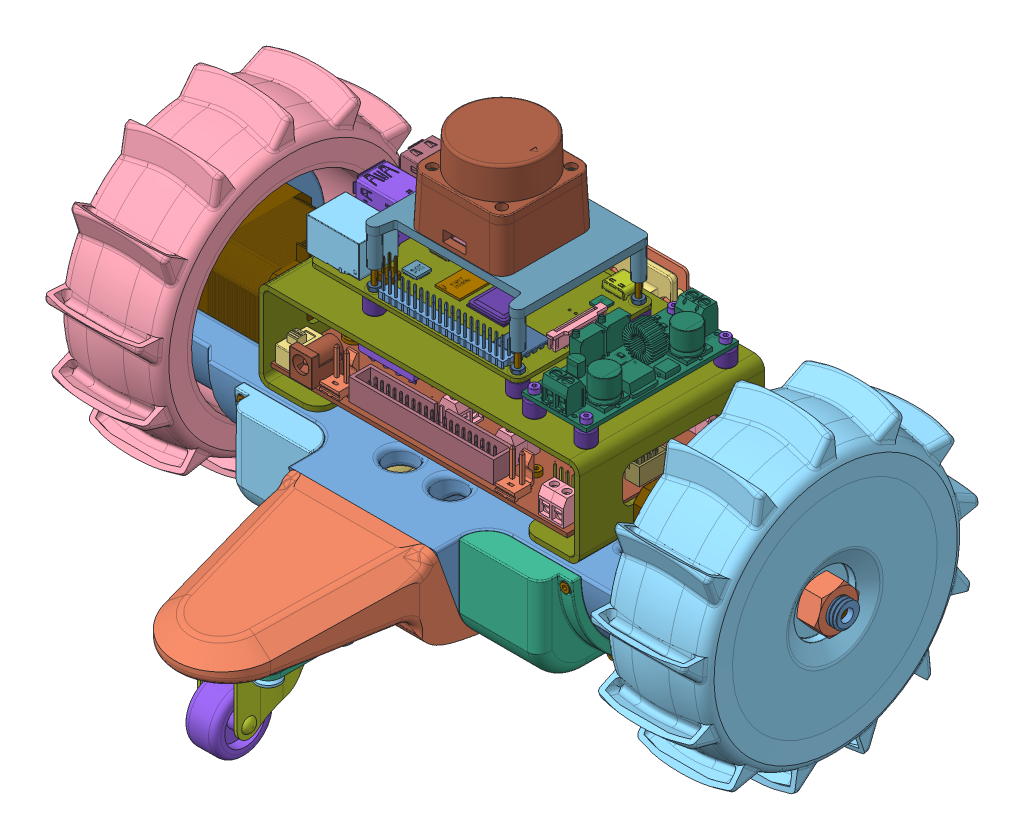
SolidWorks assembly RILeyV2_Assembly, configuration Default. Lengths in mm. (continued)
Components (placement in the parent): (continued)
- hex nut style 1 gradeab_iso-8: hex nut style 1 gradeab_iso [ISO - 4032 - M3 - W - C] at (300.5332 207.7689 553.3328) x (1 0 0) z (0 1 0) size (5.5 6.35 2.4)
- socket countersunk head screw_iso-2: socket countersunk head screw_iso [ISO 10642 - M5 x 10 - 10C] at (238.0332 177.1861 610.0431) x (0 1 0) z (-0.9954 0 -0.095805) size (10 9.43 9.43)
- socket countersunk head screw_iso-3: socket countersunk head screw_iso [ISO 10642 - M5 x 10 - 10C] at (238.0332 177.1861 639.0431) x (0 1 0) z (-0.549026 0 0.835805) size (10 9.43 9.43)
- socket countersunk head screw_iso-4: socket countersunk head screw_iso [ISO 10642 - M5 x 10 - 10C] at (267.0332 177.1861 639.0431) x (0 1 0) z (-0.752778 0 -0.658274) size (10 9.43 9.43)
- socket countersunk head screw_iso-5: socket countersunk head screw_iso [ISO 10642 - M5 x 10 - 10C] at (267.0332 177.1861 610.0431) x (0 1 0) z (-0.538139 0 0.842856) size (10 9.43 9.43)
Mates (geometry in assembly coordinates):
- Coincident1: coincident aligned: plane of MiddlepartV2-1 through (252.5332 203.3689 525.8328) normal (0 1 0); plane of MiddlepartTailV2-1 through (282.5332 203.3689 577.1871) normal (0 1 0)
- Coincident4: coincident anti-aligned: line of MiddlepartV2-1 through (223.5332 203.3689 586.6171) axis (1 0 0); line of MiddlepartTailV2-1 through (278.0554 203.3689 586.6171) axis (-1 0 0)
- Width1: width anti-aligned: plane of MiddlepartTailV2-1 through (283.4552 145.3689 587.849) normal (0.985029 0 0.172389); plane of MiddlepartV2-1 through (219.8281 145.3689 577.6605) normal (-0.985029 0 0.172389); plane of MiddlepartTailV2-1 through (282.5332 203.3689 670.8328) normal (1 0 0); plane of MiddlepartV2-1 through (222.5332 203.3689 670.8328) normal (-1 0 0)
- Coincident6: coincident anti-aligned: plane of swifflewheel-1 through (31.0041 112.5645 302.2353) normal (0 1 0); plane of MiddlepartTailV2-1 through (222.5332 182.3689 577.1871) normal (0 -1 0)
- Width2: width aligned: plane of swifflewheel-1 through (26.0041 112.5645 302.2353) normal (-1 0 0); plane of MiddlepartTailV2-1 through (66.0041 112.5645 302.2353) normal (1 0 0); plane of swifflewheel-1 through (283.4552 145.3689 587.849) normal (0.985029 0 0.172389); plane of MiddlepartTailV2-1 through (219.8281 145.3689 577.6605) normal (-0.985029 0 0.172389)
- Coincident8: coincident: plane of swifflewheel-1 through (31.0041 112.5645 307.2353) normal (0 0 1); line of MiddlepartTailV2-1 through (231.5332 185.8689 644.5431) axis (0 1 0)
- Concentric1: concentric aligned: circle of swifflewheel-1; circle of swifflewheelMid-1
- Coincident9: coincident anti-aligned: plane of swifflewheel-1 through (31.0041 109.0645 302.2353) normal (0 -1 0); plane of swifflewheelMid-1 through (46.0041 109.0645 287.2353) normal (0 1 0)
- Concentric2: concentric aligned: cylinder of swifflewheelMid-1 through (58.5007 88.5361 300.0351) axis (-0.952407 0 0.30483) radius 1.5; cylinder of swifflewheelwheel-1 through (-895.8822 88.5361 605.4977) axis (-0.952407 0 0.30483) radius 1.5
- Width3: width anti-aligned: plane of swifflewheelMid-1 through (36.5271 75.0645 279.7688) normal (0.952407 0 -0.30483); plane of swifflewheelwheel-1 through (49.3846 75.0645 275.6536) normal (-0.952407 0 0.30483); plane of swifflewheelMid-1 through (45.0365 87.5545 305.5354) normal (-0.952407 0 0.30483); plane of swifflewheelwheel-1 through (57.4178 87.5545 301.5726) normal (0.952407 0 -0.30483)
- Concentric3: concentric anti-aligned: circle of MiddlepartV2-1; circle of ReelyBuggyWheel_Left-1
- Concentric4: concentric anti-aligned: circle of MiddlepartV2-1; circle of ReelyBuggyWheel_Right-1
- Coincident12: coincident anti-aligned: plane of MiddlepartV2-1 through (367.5332 203.3689 525.8328) normal (1 0 0); plane of ReelyBuggyWheel_Right-1 through (161.0041 133.5645 188.525) normal (-1 0 0)
- Coincident13: coincident anti-aligned: plane of MiddlepartV2-1 through (137.5332 203.3689 525.8328) normal (-1 0 0); plane of ReelyBuggyWheel_Left-1 through (-68.9959 133.5645 188.525) normal (1 0 0)
- Concentric6: concentric aligned: cylinder of MiddlepartV2-1 through (300.5332 190.4192 498.3328) axis (0 1 0) radius 1.75; cylinder of 3rdFloor_Sheetmetal-1 through (94.0041 128.6147 161.025) axis (0 1 0) radius 1.75
- Coincident14: coincident anti-aligned: plane of MiddlepartV2-1 through (252.5332 203.3689 525.8328) normal (0 1 0); plane of 3rdFloor_Sheetmetal-1 through (46.0041 133.5645 188.525) normal (0 -1 0)
- Concentric7: concentric aligned: cylinder of MiddlepartV2-1 through (204.5332 190.4192 498.3328) axis (0 1 0) radius 1.75; cylinder of 3rdFloor_Sheetmetal-1 through (-1.9959 128.6147 161.025) axis (0 1 0) radius 1.75
- Concentric8: concentric aligned: cylinder of MiddlepartTailV2-1 through (238.0332 207.3041 610.0431) axis (0 -1 0) radius 2.3; cylinder of SwivelWheel-1/SwivelWheelBase-1 through (238.0332 182.3689 610.0431) axis (0 -1 0) radius 2.65
- Concentric10: concentric aligned: cylinder of MiddlepartTailV2-1 through (267.0332 207.3041 610.0431) axis (0 -1 0) radius 2.3; cylinder of SwivelWheel-1/SwivelWheelBase-1 through (267.0332 182.3689 610.0431) axis (0 -1 0) radius 2.65
- Coincident15: coincident anti-aligned: plane of MiddlepartTailV2-1 through (222.5332 182.3689 577.1871) normal (0 -1 0); plane of SwivelWheel-1/SwivelWheelBase-1 through (267.5332 182.3689 639.5431) normal (0 1 0)
- Concentric11: concentric aligned: cylinder of MiddlepartTailV2-1 through (238.0332 207.3041 610.0431) axis (0 -1 0) radius 2.3; cylinder of SwivelWheel-1/SwivelWheelBase-1 through (238.0332 182.3689 610.0431) axis (0 -1 0) radius 2.65
- Coincident16: coincident aligned: plane of MiddlepartTailV2-1 through (282.5332 203.3689 577.1871) normal (0 1 0); plane of MiddlepartV2-1 through (252.5332 203.3689 525.8328) normal (0 1 0)
- Coincident17: coincident anti-aligned: line of MiddlepartTailV2-1 through (278.0554 203.3689 586.6171) axis (-1 0 0); line of MiddlepartV2-1 through (223.5332 203.3689 586.6171) axis (1 0 0)
- Width4: width anti-aligned: plane of MiddlepartTailV2-1 through (283.4552 145.3689 587.849) normal (0.985029 0 0.172389); plane of MiddlepartV2-1 through (219.8281 145.3689 577.6605) normal (-0.985029 0 0.172389); plane of MiddlepartTailV2-1 through (282.5332 203.3689 670.8328) normal (1 0 0); plane of MiddlepartV2-1 through (222.5332 203.3689 670.8328) normal (-1 0 0)
- Width5: width aligned: plane of 3_battery_pack-2/link2-2 through (306.5332 181.8689 563.8328) normal (1 0 0); plane of MiddlepartV2-1 through (262.5332 178.8689 563.8328) normal (-1 0 0); plane of 3_battery_pack-2/link2-2 through (255.0332 203.3689 525.8328) normal (1 0 0); plane of MiddlepartV2-1 through (314.0332 195.3689 570.8328) normal (-1 0 0)
- Concentric12: concentric anti-aligned: cylinder of CameraAssembly-1/CameraMount-1 through (257.5332 206.8689 488.8328) axis (-1 0 0) radius 1; cylinder of MiddlepartV2-1 through (247.2805 206.8689 488.8328) axis (1 0 0) radius 1.15
- Coincident18: coincident anti-aligned: plane of 3rdFloorAssembly-1/3rdFloor_Sheetmetal-1 through (252.5332 203.3689 525.8328) normal (0 -1 0); plane of MiddlepartV2-1 through (252.5332 203.3689 525.8328) normal (0 1 0)
- Parallel1: parallel anti-aligned: plane of 3_battery_pack-2/link2-2 through (305.5332 181.8689 563.8328) normal (0 0 1); plane of MiddlepartV2-1 through (252.5332 203.3689 570.8328) normal (0 0 -1)
- Coincident19: coincident anti-aligned: plane of MiddlepartTailV2-1 through (222.5332 182.3689 577.1871) normal (0 -1 0); plane of SwivelWheel-1/SwivelWheelBase-1 through (267.5332 182.3689 639.5431) normal (0 1 0)
- Tangent1: tangent anti-aligned: cylinder of 3_battery_pack-2/Li-ion Battery-3 through (302.5332 180.3689 563.6328) axis (0 0 1) radius 9; plane of MiddlepartV2-1 through (191.0332 171.3689 570.8328) normal (0 1 0)
- Distance1: distance = 7 mm anti-aligned: plane of 3_battery_pack-2/link2-2 through (305.5332 181.8689 563.8328) normal (0 0 1); plane of MiddlepartV2-1 through (252.5332 203.3689 570.8328) normal (0 0 -1)
- Tangent2: tangent anti-aligned: cylinder of 3_battery_pack-2/Li-ion Battery-1 through (266.5332 180.3689 563.6328) axis (0 0 1) radius 9; plane of MiddlepartV2-1 through (191.0332 171.3689 570.8328) normal (0 1 0)
- Tangent3: tangent anti-aligned: cylinder of 3_battery_pack-1/Li-ion Battery-1 through (202.5332 180.3689 563.6328) axis (0 0 1) radius 9; plane of MiddlepartV2-1 through (191.0332 171.3689 570.8328) normal (0 1 0)
- Concentric13: concentric aligned: cylinder of MiddlepartTailV2-1 through (267.0332 207.3041 610.0431) axis (0 -1 0) radius 2.3; cylinder of SwivelWheel-1/SwivelWheelBase-1 through (267.0332 182.3689 610.0431) axis (0 -1 0) radius 2.65
- Concentric14: concentric aligned: cylinder of 3rdFloorAssembly-1/3rdFloor_Sheetmetal-1 through (204.5332 198.4192 498.3328) axis (0 1 0) radius 1.75; cylinder of MiddlepartV2-1 through (204.5332 190.4192 498.3328) axis (0 1 0) radius 1.75
- Concentric15: concentric aligned: cylinder of 3rdFloorAssembly-1/3rdFloor_Sheetmetal-1 through (300.5332 198.4192 498.3328) axis (0 1 0) radius 1.75; cylinder of MiddlepartV2-1 through (300.5332 190.4192 498.3328) axis (0 1 0) radius 1.75
- Width6: width anti-aligned: plane of TimeOfFlightAssembly-1/TimeOfFlightMount-1 through (250.2832 209.093 471.0696) normal (1 0 0); plane of MiddlepartV2-1 through (254.7832 209.093 471.0696) normal (-1 0 0); plane of TimeOfFlightAssembly-1/TimeOfFlightMount-1 through (254.5332 203.3689 525.8328) normal (1 0 0); plane of MiddlepartV2-1 through (250.5332 203.3689 525.8328) normal (-1 0 0)
- Distance2: distance = 7 mm anti-aligned: plane of 3_battery_pack-1/link2-2 through (241.5332 181.8689 563.8328) normal (0 0 1); plane of MiddlepartV2-1 through (252.5332 203.3689 570.8328) normal (0 0 -1)
- Concentric16: concentric aligned: cylinder of TimeOfFlightAssembly-1/TimeOfFlightMount-1 through (244.2805 202.3689 482.3328) axis (1 0 0) radius 1.15; cylinder of MiddlepartV2-1 through (247.2805 202.3689 482.3328) axis (1 0 0) radius 1.15
- Tangent4: tangent anti-aligned: cylinder of 3_battery_pack-1/Li-ion Battery-3 through (238.5332 180.3689 563.6328) axis (0 0 1) radius 9; plane of MiddlepartV2-1 through (191.0332 171.3689 570.8328) normal (0 1 0)
- Width7: width anti-aligned: plane of CameraAssembly-1/CameraMount-1 through (254.7832 204.1451 506.8767) normal (-1 0 0); plane of MiddlepartV2-1 through (250.2832 204.1451 506.8767) normal (1 0 0); plane of CameraAssembly-1/CameraMount-1 through (254.5332 203.3689 525.8328) normal (1 0 0); plane of MiddlepartV2-1 through (250.5332 203.3689 525.8328) normal (-1 0 0)
- Concentric17: concentric anti-aligned: cylinder of BatteryCoverFront-1 through (184.0332 203.3689 525.8328) axis (1 0 0) radius 40; cylinder of MiddlepartV2-1 through (367.5332 203.3689 525.8328) axis (-1 0 0) radius 40
- Parallel2: parallel anti-aligned: plane of 3_battery_pack-1/link2-2 through (241.5332 181.8689 563.8328) normal (0 0 1); plane of MiddlepartV2-1 through (252.5332 203.3689 570.8328) normal (0 0 -1)
- Parallel3: parallel anti-aligned: plane of 3_battery_pack-1/link2-2 through (198.5332 178.8689 563.8328) normal (-1 0 0); plane of MiddlepartV2-1 through (191.0332 195.3689 570.8328) normal (1 0 0)
- Parallel4: parallel anti-aligned: plane of 3_battery_pack-2/link2-2 through (306.5332 181.8689 563.8328) normal (1 0 0); plane of MiddlepartV2-1 through (314.0332 195.3689 570.8328) normal (-1 0 0)
- Concentric18: concentric aligned: cylinder of BatteryCoverBackLeft-1 through (222.5332 203.3689 525.8328) axis (-1 0 0) radius 40; cylinder of MiddlepartV2-1 through (367.5332 203.3689 525.8328) axis (-1 0 0) radius 40
- Width8: width aligned: plane of 3_battery_pack-1/link2-2 through (242.5332 181.8689 563.8328) normal (1 0 0); plane of MiddlepartV2-1 through (198.5332 178.8689 563.8328) normal (-1 0 0); plane of 3_battery_pack-1/link2-2 through (191.0332 195.3689 570.8328) normal (1 0 0); plane of MiddlepartV2-1 through (250.0332 203.3689 525.8328) normal (-1 0 0)
- Concentric19: concentric aligned: cylinder of BatteryCoverFront-1 through (187.0332 199.8689 481.8328) axis (0 0 1) radius 1; cylinder of MiddlepartV2-1 through (187.0332 199.8689 475.8328) axis (0 0 1) radius 1
- Concentric20: concentric aligned: cylinder of BatteryCoverFront-1 through (318.0332 199.8689 481.8328) axis (0 0 1) radius 1; cylinder of MiddlepartV2-1 through (318.0332 199.8689 475.8328) axis (0 0 1) radius 1
- Concentric21: concentric aligned: cylinder of BatteryCoverBackRight-1 through (318.0332 166.8689 577.4) axis (0 0 -1) radius 1; cylinder of MiddlepartV2-1 through (318.0332 166.8689 550.8328) axis (0 0 -1) radius 1
- Concentric22: concentric aligned: cylinder of BatteryCoverBackRight-1 through (282.5332 203.3689 525.8328) axis (-1 0 0) radius 40; cylinder of MiddlepartV2-1 through (367.5332 203.3689 525.8328) axis (-1 0 0) radius 40
- Concentric23: concentric aligned: cylinder of RILey_PCB_V2-1/RILey-PCB_V2.0.step-1/Board.step-1 through (285.3832 212.1009 548.6828) axis (0 -1 0) radius 1.4; cylinder of MiddlepartV2-1 through (285.3832 211.3689 548.6828) axis (0 -1 0) radius 1
- Concentric24: concentric aligned: cylinder of BatteryCoverBackLeft-1 through (187.0332 166.8689 577.4) axis (0 0 -1) radius 1; cylinder of MiddlepartV2-1 through (187.0332 166.8689 550.8328) axis (0 0 -1) radius 1
- Coincident20: coincident anti-aligned: plane of RILey_PCB_V2-1/RILey-PCB_V2.0.step-1/Board.step-1 through (252.5332 211.3689 528.3328) normal (0 -1 0); plane of MiddlepartV2-1 through (285.3832 211.3689 502.9828) normal (0 1 0)
- Concentric25: concentric aligned: cylinder of BatteryCoverBackLeft-1 through (187.0332 199.8689 577.4) axis (0 0 -1) radius 1; cylinder of MiddlepartV2-1 through (187.0332 199.8689 575.8328) axis (0 0 -1) radius 1
- Concentric26: concentric aligned: cylinder of BatteryCoverBackRight-1 through (318.0332 199.8689 577.4) axis (0 0 -1) radius 1; cylinder of MiddlepartV2-1 through (318.0332 199.8689 575.8328) axis (0 0 -1) radius 1
- Concentric27: concentric aligned: cylinder of RILey_PCB_V2-1/RILey-PCB_V2.0.step-1/Board.step-1 through (285.3832 212.1009 502.9828) axis (0 -1 0) radius 1.4; cylinder of MiddlepartV2-1 through (285.3832 211.3689 502.9828) axis (0 -1 0) radius 1
- Coincident21: coincident anti-aligned: plane of MiddlepartV2-1 through (142.5332 243.3689 485.8328) normal (1 0 0); plane of Nema_17-17HS4401.step-2/eBom-FreeParts-1 through (142.5332 203.3689 525.8328) normal (-1 0 0)
- Concentric30: concentric anti-aligned: cylinder of MiddlepartV2-1 through (148.19 187.8689 541.3328) axis (-1 0 0) radius 2; cylinder of Nema_17-17HS4401.step-2/eBom-FreeParts-1 through (142.5332 187.8689 541.3328) axis (1 0 0) radius 1.25
- Concentric31: concentric anti-aligned: cylinder of MiddlepartV2-1 through (148.19 218.8689 541.3328) axis (-1 0 0) radius 2; cylinder of Nema_17-17HS4401.step-2/eBom-FreeParts-1 through (142.5332 218.8689 541.3328) axis (1 0 0) radius 1.25
- Concentric32: concentric anti-aligned: cylinder of MiddlepartV2-1 through (356.8763 218.8689 541.3328) axis (1 0 0) radius 2; cylinder of Nema_17-17HS4401.step-1/eBom-FreeParts-1 through (362.5332 218.8689 541.3328) axis (-1 0 0) radius 1.25
- Concentric33: concentric anti-aligned: cylinder of MiddlepartV2-1 through (356.8763 218.8689 510.3328) axis (1 0 0) radius 2; cylinder of Nema_17-17HS4401.step-1/eBom-FreeParts-1 through (362.5332 218.8689 510.3328) axis (-1 0 0) radius 1.25
- Coincident22: coincident anti-aligned: plane of MiddlepartV2-1 through (362.5332 243.3689 485.8328) normal (-1 0 0); plane of Nema_17-17HS4401.step-1/eBom-FreeParts-1 through (362.5332 203.3689 525.8328) normal (1 0 0)
- Concentric34: concentric aligned: cylinder of Nema_17-17HS4401.step-1/eBom-FreeParts-1 through (386.1082 203.3689 525.8328) axis (-1 0 0) radius 2.5; cylinder of RightWheelAssembly-1/HexBolt_modified-1 through (395.6043 203.3689 525.8328) axis (-1 0 0) radius 2.5
- Parallel5: parallel aligned: plane of Nema_17-17HS4401.step-1/eBom-FreeParts-1 through (368.6082 205.3689 -4474.1672) normal (0 1 0); plane of RightWheelAssembly-1/HexBolt_modified-1 through (373.5332 211.8689 520.9254) normal (0 1 0)
- Coincident24: coincident anti-aligned: plane of MiddlepartV2-1 through (367.5332 203.3689 525.8328) normal (1 0 0); plane of RightWheelAssembly-1/HexBolt_modified-1 through (367.5332 203.3689 525.8328) normal (-1 0 0)
- Concentric35: concentric aligned: cylinder of Nema_17-17HS4401.step-2/eBom-FreeParts-1 through (118.9582 203.3689 525.8328) axis (1 0 0) radius 2.5; cylinder of LeftWheelAssembly-1/HexBolt_modified-1 through (109.4621 203.3689 525.8328) axis (1 0 0) radius 2.5
- Parallel6: parallel aligned: plane of Nema_17-17HS4401.step-2/eBom-FreeParts-1 through (136.4582 205.3689 5525.8328) normal (0 1 0); plane of LeftWheelAssembly-1/HexBolt_modified-1 through (131.5332 211.8689 530.7403) normal (0 1 0)
- Coincident26: coincident anti-aligned: plane of MiddlepartV2-1 through (137.5332 203.3689 525.8328) normal (-1 0 0); plane of LeftWheelAssembly-1/HexBolt_modified-1 through (137.5332 203.3689 525.8328) normal (1 0 0)
- Concentric36: concentric aligned: cylinder of BatteryCoverFront-1 through (187.0332 199.8689 483.8328) axis (0 0 -1) radius 2; cylinder of socket head cap screw_iso-2 through (187.0332 199.8689 450.0828) axis (0 0 -1) radius 1.9
- Coincident27: coincident anti-aligned: plane of BatteryCoverFront-1 through (187.0332 199.8689 483.8328) normal (0 0 -1); plane of socket head cap screw_iso-2 through (187.0332 201.7689 483.8328) normal (0 0 1)
- Concentric37: concentric aligned: cylinder of BatteryCoverFront-1 through (318.0332 199.8689 483.8328) axis (0 0 -1) radius 2; cylinder of socket head cap screw_iso-3 through (318.0332 199.8689 450.0828) axis (0 0 -1) radius 1.9
- Coincident28: coincident anti-aligned: plane of BatteryCoverFront-1 through (318.0332 199.8689 483.8328) normal (0 0 -1); plane of socket head cap screw_iso-3 through (318.0332 201.7689 483.8328) normal (0 0 1)
- Concentric38: concentric aligned: cylinder of BatteryCoverBackLeft-1 through (187.0332 199.8689 567.9) axis (0 0 1) radius 2; cylinder of socket head cap screw_iso-4 through (187.0332 199.8689 601.65) axis (0 0 1) radius 1.9
- Coincident29: coincident anti-aligned: plane of BatteryCoverBackLeft-1 through (187.0332 199.8689 567.9) normal (0 0 1); plane of socket head cap screw_iso-4 through (187.0332 201.7689 567.9) normal (0 0 -1)
- Concentric39: concentric aligned: cylinder of BatteryCoverBackRight-1 through (318.0332 199.8689 567.9) axis (0 0 1) radius 2; cylinder of socket head cap screw_iso-5 through (318.0332 199.8689 601.65) axis (0 0 1) radius 1.9
- Coincident30: coincident anti-aligned: plane of BatteryCoverBackRight-1 through (318.0332 199.8689 567.9) normal (0 0 1); plane of socket head cap screw_iso-5 through (318.0332 201.7689 567.9) normal (0 0 -1)
- Concentric40: concentric aligned: cylinder of BatteryCoverBackLeft-1 through (187.0332 166.8689 548.9) axis (0 0 1) radius 2; cylinder of socket head cap screw_iso-7 through (187.0332 166.8689 582.65) axis (0 0 1) radius 1.9
- Coincident31: coincident anti-aligned: plane of BatteryCoverBackLeft-1 through (187.0332 166.8689 548.9) normal (0 0 1); plane of socket head cap screw_iso-7 through (187.0332 168.7689 548.9) normal (0 0 -1)
- Concentric41: concentric aligned: cylinder of BatteryCoverBackRight-1 through (318.0332 166.8689 548.9) axis (0 0 1) radius 2; cylinder of socket head cap screw_iso-8 through (318.0332 166.8689 582.65) axis (0 0 1) radius 1.9
- Coincident32: coincident anti-aligned: plane of BatteryCoverBackRight-1 through (318.0332 166.8689 548.9) normal (0 0 1); plane of socket head cap screw_iso-8 through (318.0332 168.7689 548.9) normal (0 0 -1)
- Concentric42: concentric anti-aligned: cylinder of BatteryCoverFront-1 through (318.0332 166.8689 497.8328) axis (0 0 1) radius 2; cylinder of socket head cap screw_iso-9 through (318.0332 166.8689 470.0828) axis (0 0 -1) radius 1.9
- Coincident33: coincident anti-aligned: plane of BatteryCoverFront-1 through (318.0332 166.8689 503.8328) normal (0 0 -1); plane of socket head cap screw_iso-9 through (318.0332 168.7689 503.8328) normal (0 0 1)
- Concentric43: concentric anti-aligned: cylinder of BatteryCoverFront-1 through (252.5332 166.8689 497.8328) axis (0 0 1) radius 2; cylinder of socket head cap screw_iso-10 through (252.5332 166.8689 470.0828) axis (0 0 -1) radius 1.9
- Coincident34: coincident anti-aligned: plane of BatteryCoverFront-1 through (252.5332 166.8689 503.8328) normal (0 0 -1); plane of socket head cap screw_iso-10 through (252.5332 168.7689 503.8328) normal (0 0 1)
- Concentric44: concentric anti-aligned: cylinder of BatteryCoverFront-1 through (187.0332 166.8689 497.8328) axis (0 0 1) radius 2; cylinder of socket head cap screw_iso-11 through (187.0332 166.8689 470.0828) axis (0 0 -1) radius 1.9
- Coincident35: coincident anti-aligned: plane of BatteryCoverFront-1 through (187.0332 166.8689 503.8328) normal (0 0 -1); plane of socket head cap screw_iso-11 through (187.0332 168.7689 503.8328) normal (0 0 1)
- Concentric45: concentric anti-aligned: cylinder of MiddlepartV2-1 through (233.5332 188.3689 560.8328) axis (0 0 1) radius 4.35; cylinder of socket head cap screw_iso-14 through (233.5332 188.3689 538.0828) axis (0 0 -1) radius 4.25
- Coincident36: coincident anti-aligned: plane of MiddlepartV2-1 through (233.5332 188.3689 574.8328) normal (0 0 -1); plane of socket head cap screw_iso-14 through (233.5332 192.6189 574.8328) normal (0 0 1)
- Concentric46: concentric aligned: cylinder of MiddlepartV2-1 through (271.5332 188.3689 586.6171) axis (0 0 -1) radius 2.65; cylinder of socket head cap screw_iso-15 through (271.5332 188.3689 538.0828) axis (0 0 -1) radius 4.25
- Coincident37: coincident anti-aligned: plane of MiddlepartV2-1 through (271.5332 188.3689 574.8328) normal (0 0 -1); plane of socket head cap screw_iso-15 through (271.5332 192.6189 574.8328) normal (0 0 1)
- Concentric47: concentric anti-aligned: cylinder of RILey_PCB_V2-1/RILey-PCB_V2.0.step-1/Board.step-1 through (219.6832 212.1009 502.9828) axis (0 -1 0) radius 1.4; cylinder of socket head cap screw_iso-17 through (219.6832 246.6889 502.9828) axis (0 1 0) radius 1.9
- Coincident38: coincident anti-aligned: plane of RILey_PCB_V2-1/RILey-PCB_V2.0.step-1/Board.step-1 through (252.5332 212.9389 528.3328) normal (0 1 0); plane of socket head cap screw_iso-17 through (221.5832 212.9389 502.9828) normal (0 -1 0)
- Concentric48: concentric anti-aligned: cylinder of RILey_PCB_V2-1/RILey-PCB_V2.0.step-1/Board.step-1 through (285.3832 212.1009 502.9828) axis (0 -1 0) radius 1.4; cylinder of socket head cap screw_iso-18 through (285.3832 246.6889 502.9828) axis (0 1 0) radius 1.9
- Coincident39: coincident anti-aligned: plane of RILey_PCB_V2-1/RILey-PCB_V2.0.step-1/Board.step-1 through (252.5332 212.9389 528.3328) normal (0 1 0); plane of socket head cap screw_iso-18 through (287.2832 212.9389 502.9828) normal (0 -1 0)
- Concentric49: concentric anti-aligned: cylinder of RILey_PCB_V2-1/RILey-PCB_V2.0.step-1/Board.step-1 through (219.6832 212.1009 548.6828) axis (0 -1 0) radius 1.4; cylinder of socket head cap screw_iso-19 through (219.6832 246.6889 548.6828) axis (0 1 0) radius 1.9
- Coincident40: coincident anti-aligned: plane of RILey_PCB_V2-1/RILey-PCB_V2.0.step-1/Board.step-1 through (252.5332 212.9389 528.3328) normal (0 1 0); plane of socket head cap screw_iso-19 through (221.5832 212.9389 548.6828) normal (0 -1 0)
- Concentric50: concentric anti-aligned: cylinder of RILey_PCB_V2-1/RILey-PCB_V2.0.step-1/Board.step-1 through (285.3832 212.1009 548.6828) axis (0 -1 0) radius 1.4; cylinder of socket head cap screw_iso-20 through (285.3832 246.6889 548.6828) axis (0 1 0) radius 1.9
- Coincident41: coincident anti-aligned: plane of RILey_PCB_V2-1/RILey-PCB_V2.0.step-1/Board.step-1 through (252.5332 212.9389 528.3328) normal (0 1 0); plane of socket head cap screw_iso-20 through (287.2832 212.9389 548.6828) normal (0 -1 0)
- Concentric51: concentric aligned: cylinder of MiddlepartV2-1 through (300.5332 198.3689 553.3328) axis (0 -1 0) radius 2.95; cylinder of socket head cap screw_iso-22 through (300.5332 163.6189 553.3328) axis (0 -1 0) radius 2.75
- Coincident42: coincident anti-aligned: plane of MiddlepartV2-1 through (300.5332 198.3689 553.3328) normal (0 -1 0); plane of socket head cap screw_iso-22 through (297.7832 198.3689 553.3328) normal (0 1 0)
- Concentric52: concentric anti-aligned: cylinder of MiddlepartV2-1 through (300.5332 190.4192 553.3328) axis (0 1 0) radius 1.75; cylinder of socket head cap screw_iso-24 through (300.5332 163.6189 553.3328) axis (0 -1 0) radius 2.75
- Coincident43: coincident anti-aligned: plane of MiddlepartV2-1 through (300.5332 198.3689 553.3328) normal (0 -1 0); plane of socket head cap screw_iso-24 through (297.7832 198.3689 553.3328) normal (0 1 0)
- Concentric53: concentric anti-aligned: cylinder of MiddlepartV2-1 through (204.5332 190.4192 553.3328) axis (0 1 0) radius 1.75; cylinder of socket head cap screw_iso-25 through (204.5332 163.6189 553.3328) axis (0 -1 0) radius 2.75
- Coincident44: coincident anti-aligned: plane of MiddlepartV2-1 through (204.5332 198.3689 553.3328) normal (0 -1 0); plane of socket head cap screw_iso-25 through (201.7832 198.3689 553.3328) normal (0 1 0)
- Concentric54: concentric anti-aligned: cylinder of MiddlepartV2-1 through (204.5332 190.4192 498.3328) axis (0 1 0) radius 1.75; cylinder of socket head cap screw_iso-26 through (204.5332 163.6189 498.3328) axis (0 -1 0) radius 2.75
- Coincident45: coincident anti-aligned: plane of MiddlepartV2-1 through (204.5332 198.3689 498.3328) normal (0 -1 0); plane of socket head cap screw_iso-26 through (201.7832 198.3689 498.3328) normal (0 1 0)
- Concentric55: concentric anti-aligned: cylinder of MiddlepartV2-1 through (300.5332 190.4192 498.3328) axis (0 1 0) radius 1.75; cylinder of socket head cap screw_iso-27 through (300.5332 163.6189 498.3328) axis (0 -1 0) radius 2.75
- Coincident46: coincident anti-aligned: plane of MiddlepartV2-1 through (300.5332 198.3689 498.3328) normal (0 -1 0); plane of socket head cap screw_iso-27 through (297.7832 198.3689 498.3328) normal (0 1 0)
- Coincident47: coincident anti-aligned: plane of CameraAssembly-1/CameraMount-1 through (257.5332 209.5927 470.789) normal (1 0 0); plane of socket head cap screw_iso-29 through (257.5332 207.5944 487.0768) normal (-1 0 0)
- Concentric56: concentric anti-aligned: cylinder of CameraAssembly-1/CameraMount-1 through (257.5332 206.8689 488.8328) axis (-1 0 0) radius 1; cylinder of socket head cap screw_iso-29 through (291.2832 206.8689 488.8328) axis (1 0 0) radius 1
- Concentric57: concentric anti-aligned: cylinder of TimeOfFlightAssembly-1/TimeOfFlightMount-1 through (244.2805 202.3689 482.3328) axis (1 0 0) radius 1.15; cylinder of socket head cap screw_iso-28 through (213.7832 202.3689 482.3328) axis (-1 0 0) radius 1
- Coincident48: coincident anti-aligned: plane of TimeOfFlightAssembly-1/TimeOfFlightMount-1 through (247.5332 205.8857 482.6963) normal (-1 0 0); plane of socket head cap screw_iso-28 through (247.5332 202.3127 480.4337) normal (1 0 0)
- Concentric58: concentric aligned: cylinder of MiddlepartV2-1 through (365.0332 218.8689 510.3328) axis (1 0 0) radius 3; cylinder of socket head cap screw_iso-32 through (399.7832 218.8689 510.3328) axis (1 0 0) radius 2.75
- Coincident49: coincident anti-aligned: plane of MiddlepartV2-1 through (365.0332 218.8689 510.3328) normal (1 0 0); plane of socket head cap screw_iso-32 through (365.0332 217.8188 512.8745) normal (-1 0 0)
- Concentric59: concentric aligned: cylinder of MiddlepartV2-1 through (356.8763 218.8689 541.3328) axis (1 0 0) radius 2; cylinder of socket head cap screw_iso-33 through (399.7832 218.8689 541.3328) axis (1 0 0) radius 2.75
- Coincident50: coincident anti-aligned: plane of MiddlepartV2-1 through (365.0332 218.8689 541.3328) normal (1 0 0); plane of socket head cap screw_iso-33 through (365.0332 217.8188 543.8745) normal (-1 0 0)
- Concentric60: concentric aligned: cylinder of MiddlepartV2-1 through (356.8763 187.8689 541.3328) axis (1 0 0) radius 2; cylinder of socket head cap screw_iso-34 through (399.7832 187.8689 541.3328) axis (1 0 0) radius 2.75
- Coincident51: coincident anti-aligned: plane of MiddlepartV2-1 through (365.0332 187.8689 541.3328) normal (1 0 0); plane of socket head cap screw_iso-34 through (365.0332 186.8188 543.8745) normal (-1 0 0)
- Concentric61: concentric aligned: cylinder of MiddlepartV2-1 through (356.8763 187.8689 510.3328) axis (1 0 0) radius 2; cylinder of socket head cap screw_iso-35 through (399.7832 187.8689 510.3328) axis (1 0 0) radius 2.75
- Coincident52: coincident anti-aligned: plane of MiddlepartV2-1 through (365.0332 187.8689 510.3328) normal (1 0 0); plane of socket head cap screw_iso-35 through (365.0332 186.8188 512.8745) normal (-1 0 0)
- Concentric62: concentric aligned: cylinder of MiddlepartV2-1 through (140.0332 218.8689 541.3328) axis (-1 0 0) radius 3; cylinder of socket head cap screw_iso-36 through (105.2832 218.8689 541.3328) axis (-1 0 0) radius 2.75
- Coincident53: coincident anti-aligned: plane of MiddlepartV2-1 through (140.0332 218.8689 541.3328) normal (-1 0 0); plane of socket head cap screw_iso-36 through (140.0332 221.6189 541.3328) normal (1 0 0)
- Concentric63: concentric aligned: cylinder of MiddlepartV2-1 through (148.19 218.8689 510.3328) axis (-1 0 0) radius 2; cylinder of socket head cap screw_iso-37 through (105.2832 218.8689 510.3328) axis (-1 0 0) radius 2.75
- Coincident54: coincident anti-aligned: plane of MiddlepartV2-1 through (140.0332 218.8689 510.3328) normal (-1 0 0); plane of socket head cap screw_iso-37 through (140.0332 221.6189 510.3328) normal (1 0 0)
- Concentric64: concentric aligned: cylinder of MiddlepartV2-1 through (148.19 187.8689 510.3328) axis (-1 0 0) radius 2; cylinder of socket head cap screw_iso-38 through (105.2832 187.8689 510.3328) axis (-1 0 0) radius 2.75
- Coincident55: coincident anti-aligned: plane of MiddlepartV2-1 through (140.0332 187.8689 510.3328) normal (-1 0 0); plane of socket head cap screw_iso-38 through (140.0332 190.6189 510.3328) normal (1 0 0)
- Concentric65: concentric aligned: cylinder of MiddlepartV2-1 through (148.19 187.8689 541.3328) axis (-1 0 0) radius 2; cylinder of socket head cap screw_iso-39 through (105.2832 187.8689 541.3328) axis (-1 0 0) radius 2.75
- Coincident56: coincident anti-aligned: plane of MiddlepartV2-1 through (140.0332 187.8689 541.3328) normal (-1 0 0); plane of socket head cap screw_iso-39 through (140.0332 190.6189 541.3328) normal (1 0 0)
- Concentric68: concentric anti-aligned: cylinder of socket head cap screw_iso-29 through (291.2832 206.8689 488.8328) axis (1 0 0) radius 1; cylinder of hex nut style 1 gradeab_iso-3 through (247.5332 206.8689 488.8328) axis (-1 0 0) radius 0.8
- Coincident59: coincident anti-aligned: plane of CameraAssembly-1/CameraMount-1 through (247.5332 209.5927 470.789) normal (-1 0 0); plane of hex nut style 1 gradeab_iso-3 through (247.5332 204.0331 491.6539) normal (1 0 0)
- Concentric69: concentric anti-aligned: cylinder of socket head cap screw_iso-28 through (213.7832 202.3689 482.3328) axis (-1 0 0) radius 1; cylinder of hex nut style 1 gradeab_iso-2 through (257.5332 202.3689 482.3328) axis (1 0 0) radius 0.8
- Coincident60: coincident anti-aligned: plane of TimeOfFlightAssembly-1/TimeOfFlightMount-1 through (257.5332 205.8857 482.6963) normal (1 0 0); plane of hex nut style 1 gradeab_iso-2 through (257.5332 198.672 480.8054) normal (-1 0 0)
- Concentric70: concentric aligned: cylinder of 3rdFloorAssembly-1/3rdFloor_Sheetmetal-1 through (204.5332 198.4192 498.3328) axis (0 1 0) radius 1.75; cylinder of hex nut style 1 gradeab_iso-5 through (204.5332 182.7314 498.3328) axis (0 1 0) radius 1.5
- Coincident61: coincident anti-aligned: plane of 3rdFloorAssembly-1/3rdFloor_Sheetmetal-1 through (252.5332 205.3689 525.8328) normal (0 1 0); plane of hex nut style 1 gradeab_iso-5 through (204.5332 205.3689 495.1574) normal (0 -1 0)
- Concentric71: concentric aligned: cylinder of 3rdFloorAssembly-1/3rdFloor_Sheetmetal-1 through (300.5332 198.4192 498.3328) axis (0 1 0) radius 1.75; cylinder of hex nut style 1 gradeab_iso-6 through (300.5332 182.7314 498.3328) axis (0 1 0) radius 1.5
- Coincident62: coincident anti-aligned: plane of 3rdFloorAssembly-1/3rdFloor_Sheetmetal-1 through (252.5332 205.3689 525.8328) normal (0 1 0); plane of hex nut style 1 gradeab_iso-6 through (300.5332 205.3689 495.1574) normal (0 -1 0)
- Concentric72: concentric aligned: cylinder of 3rdFloorAssembly-1/3rdFloor_Sheetmetal-1 through (204.5332 198.4192 553.3328) axis (0 1 0) radius 1.75; cylinder of hex nut style 1 gradeab_iso-7 through (204.5332 182.7314 553.3328) axis (0 1 0) radius 1.5
- Coincident63: coincident anti-aligned: plane of 3rdFloorAssembly-1/3rdFloor_Sheetmetal-1 through (252.5332 205.3689 525.8328) normal (0 1 0); plane of hex nut style 1 gradeab_iso-7 through (204.5332 205.3689 550.1574) normal (0 -1 0)
- Concentric73: concentric aligned: cylinder of 3rdFloorAssembly-1/3rdFloor_Sheetmetal-1 through (300.5332 198.4192 553.3328) axis (0 1 0) radius 1.75; cylinder of hex nut style 1 gradeab_iso-8 through (300.5332 182.7314 553.3328) axis (0 1 0) radius 1.5
- Coincident64: coincident anti-aligned: plane of 3rdFloorAssembly-1/3rdFloor_Sheetmetal-1 through (252.5332 205.3689 525.8328) normal (0 1 0); plane of hex nut style 1 gradeab_iso-8 through (300.5332 205.3689 550.1574) normal (0 -1 0)
- Concentric74: concentric aligned: cylinder of SwivelWheel-1/SwivelWheelBase-1 through (238.0332 182.3689 639.0431) axis (0 -1 0) radius 2.65; cylinder of hex screw gradeab_iso-2 through (238.0332 176.8689 639.0431) axis (0 -1 0) radius 4
- Coincident65: coincident anti-aligned: plane of SwivelWheel-1/SwivelWheelBase-1 through (267.5332 180.3689 639.5431) normal (0 -1 0); plane of hex screw gradeab_iso-2 through (233.4144 180.3689 639.0431) normal (0 1 0)
- Concentric75: concentric aligned: cylinder of SwivelWheel-1/SwivelWheelBase-1 through (238.0332 182.3689 610.0431) axis (0 -1 0) radius 2.65; cylinder of hex screw gradeab_iso-3 through (238.0332 176.8689 610.0431) axis (0 -1 0) radius 4
- Coincident66: coincident anti-aligned: plane of SwivelWheel-1/SwivelWheelBase-1 through (267.5332 180.3689 639.5431) normal (0 -1 0); plane of hex screw gradeab_iso-3 through (233.4144 180.3689 610.0431) normal (0 1 0)
- Concentric76: concentric aligned: cylinder of SwivelWheel-1/SwivelWheelBase-1 through (267.0332 182.3689 610.0431) axis (0 -1 0) radius 2.65; cylinder of hex screw gradeab_iso-4 through (267.0332 176.8689 610.0431) axis (0 -1 0) radius 4
- Coincident67: coincident anti-aligned: plane of SwivelWheel-1/SwivelWheelBase-1 through (267.5332 180.3689 639.5431) normal (0 -1 0); plane of hex screw gradeab_iso-4 through (262.4144 180.3689 610.0431) normal (0 1 0)
- Concentric77: concentric aligned: cylinder of SwivelWheel-1/SwivelWheelBase-1 through (267.0332 182.3689 639.0431) axis (0 -1 0) radius 2.65; cylinder of hex screw gradeab_iso-5 through (267.0332 176.8689 639.0431) axis (0 -1 0) radius 4
- Coincident68: coincident anti-aligned: plane of SwivelWheel-1/SwivelWheelBase-1 through (267.5332 180.3689 639.5431) normal (0 -1 0); plane of hex screw gradeab_iso-5 through (262.4144 180.3689 639.0431) normal (0 1 0)
- Concentric78: concentric aligned: cylinder of MiddlepartTailV2-1 through (238.0332 207.3041 610.0431) axis (0 -1 0) radius 2.3; cylinder of socket countersunk head screw_iso-2 through (238.0332 177.1861 610.0431) axis (0 -1 0) radius 2.5
- Concentric79: concentric aligned: cylinder of MiddlepartTailV2-1 through (238.0332 207.3041 639.0431) axis (0 -1 0) radius 2.3; cylinder of socket countersunk head screw_iso-3 through (238.0332 177.1861 639.0431) axis (0 -1 0) radius 2.5
- Concentric80: concentric aligned: cylinder of MiddlepartTailV2-1 through (267.0332 207.3041 639.0431) axis (0 -1 0) radius 2.3; cylinder of socket countersunk head screw_iso-4 through (267.0332 177.1861 639.0431) axis (0 -1 0) radius 2.5
- Concentric81: concentric aligned: cylinder of MiddlepartTailV2-1 through (267.0332 207.3041 610.0431) axis (0 -1 0) radius 2.3; cylinder of socket countersunk head screw_iso-5 through (267.0332 177.1861 610.0431) axis (0 -1 0) radius 2.5
- Distance3: distance = 3.1828 mm aligned: plane of socket countersunk head screw_iso-2 through (238.0332 177.1861 610.0431) normal (0 -1 0); plane of SwivelWheel-1/SwivelWheelBase-1 through (267.5332 180.3689 639.5431) normal (0 -1 0)
- Distance4: distance = 3.1828 mm aligned: plane of socket countersunk head screw_iso-3 through (238.0332 177.1861 639.0431) normal (0 -1 0); plane of SwivelWheel-1/SwivelWheelBase-1 through (267.5332 180.3689 639.5431) normal (0 -1 0)
- Distance5: distance = 3.1828 mm aligned: plane of socket countersunk head screw_iso-4 through (267.0332 177.1861 639.0431) normal (0 -1 0); plane of SwivelWheel-1/SwivelWheelBase-1 through (267.5332 180.3689 639.5431) normal (0 -1 0)
- Distance6: distance = 3.1828 mm aligned: plane of socket countersunk head screw_iso-5 through (267.0332 177.1861 610.0431) normal (0 -1 0); plane of SwivelWheel-1/SwivelWheelBase-1 through (267.5332 180.3689 639.5431) normal (0 -1 0)
